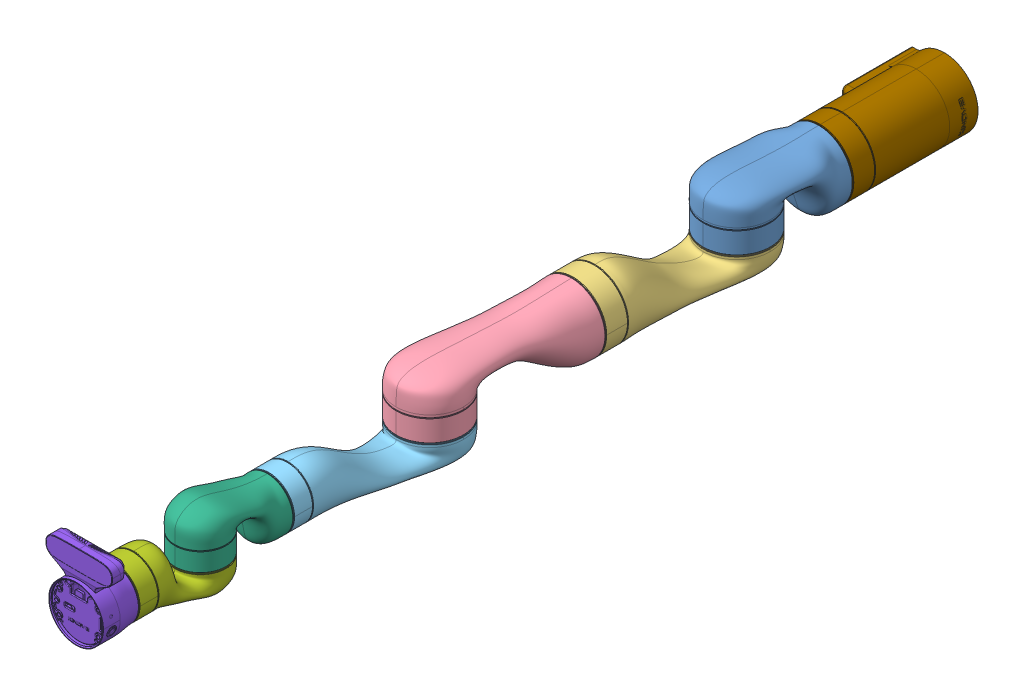
SolidWorks assembly GEN3_STEP_ARM_V11, configuration 默认. Lengths in mm.
Overall size (97.47 134.56 1190.25).
26 component instances, 10 part files, 0 mates.
Components (placement in the parent):
- GEN3_STEP_ARM_V11.STEP-1: GEN3_STEP_ARM_V11.STEP [默认] at origin size (97.47 134.56 1190.25)
  - GEN3 SIMPLIFIED SHOULDER.STEP-1: GEN3 SIMPLIFIED SHOULDER.STEP [默认] at (0 0 158.8) x (0 0 1) z (-1 0 0) size (174.42 95.54 93.63)
    - GEN3 SIMPLIFIED SHOULDER-0.STEP-1: GEN3 SIMPLIFIED SHOULDER-0.STEP [默认] at origin size (172.05 94.81 92.82)
    - KR10643.STEP-1: KR10643.STEP [默认] at (27.725 0 0) x (0 0.982111 0.188302) z (0 -0.188302 0.982111) size (80 30.1 80)
    - KR10643.STEP-2: KR10643.STEP [默认] at (126 -5.375 0) size (80 30.1 80)
  - GEN3 SIMPLIFIED HalfArm1.STEP-1: GEN3 SIMPLIFIED HalfArm1.STEP [默认] at (0 -11.75 284.8) x (0 0 1) z (1 0 0) size (270.8 96.93 92.15)
    - GEN3 SIMPLIFIED HALF ARM 1.STEP-1: GEN3 SIMPLIFIED HALF ARM 1.STEP [默认] at origin size (270.8 96.93 92.15)
    - KR10643.STEP-1: KR10643.STEP [默认] at (0 -6.375 0) size (80 30.1 80)
    - KR10643.STEP-2: KR10643.STEP [默认] at (210.375 0 0) x (0 1 0) z (0 0 1) size (80 30.1 80)
  - GEN3 SIMPLIFIED HalfArm2.STEP-1: GEN3 SIMPLIFIED HalfArm2.STEP [默认] at (0 -11.75 705.55) x (0 0 -1) z (1 0 0) size (256.38 96.93 92.15)
    - GEN3 SIMPLIFIED HALF ARM 2.STEP-1: GEN3 SIMPLIFIED HALF ARM 2.STEP [默认] at origin size (254 96.93 92.15)
    - KR10643.STEP-1: KR10643.STEP [默认] at (210.375 0 0) x (0 0 1) z (0 -1 0) size (80 30.1 80)
    - KR10643.STEP-2: KR10643.STEP [默认] at (0 -6.375 0) x (-0.999129 0 -0.041722) z (0.041722 0 -0.999129) size (80 30.1 80)
  - GEN3 SIMPLIFIED Forearm.STEP-1: GEN3 SIMPLIFIED Forearm.STEP [默认] at (0 -24.5 705.55) x (0 0 1) z (1 0 0) size (266.9 85.27 92.04)
  - GEN3 SIMPLIFIED Spherical Wrist1.STEP-1: GEN3 SIMPLIFIED Spherical Wrist1.STEP [默认] at (0 -24.5 916.4001) x (0 0 1) z (-1 0 0) size (138.52 88.25 70.01)
    - GEN3 SIMPLIFIED WRIST 1.STEP-1: GEN3 SIMPLIFIED WRIST 1.STEP [默认] at origin size (138.52 88.25 70.01)
    - KR12943.x_t-1: KR12943.x_t [默认] at (-2.4251 0 0) x (0 -1 0) z (0 0 1)
    - KR12943.x_t-2: KR12943.x_t [默认] at (103.5 -0.1751 0)
  - GEN3 SIMPLIFIED Spherical Wrist2.STEP-1: GEN3 SIMPLIFIED Spherical Wrist2.STEP [默认] at (0 -24.8501 1123.4001) x (0 0 -1) z (-1 0 0) size (153.49 88.25 70.01)
    - GEN3 SIMPLIFIED WRIST 2.STEP-1: GEN3 SIMPLIFIED WRIST 2.STEP [默认] at origin size (153.49 88.25 70.01)
    - KR12943.x_t-1: KR12943.x_t [默认] at (103.5 -0.1751 0)
    - KR12943.x_t-2: KR12943.x_t [默认] at (-2.4251 0 0) x (0 -1 0) z (0 0 1)
  - GEN3 SIMPLIFIED Vision.STEP-1: GEN3 SIMPLIFIED Vision.STEP [默认] at (0 -24.8501 1128.3252) size (97.47 118.83 61.93)
    - GEN3 SIMPLIFIED VISION with interface NO GRIPPER NO CAP.STEP-1: GEN3 SIMPLIFIED VISION with interface NO GRIPPER NO CAP.STEP [默认] at origin size (97.47 118.83 61.93)
    - KR12943.x_t-1: KR12943.x_t [默认] at (0 0 29.5) x (0 -1 0) z (1 0 0)
  - GEN3 SIMPLIFIED BASE.STEP-1: GEN3 SIMPLIFIED BASE.STEP [默认] at (0 0 1.8) x (-1 0 0) z (0 1 0) size (92.5 170.85 92.16)
